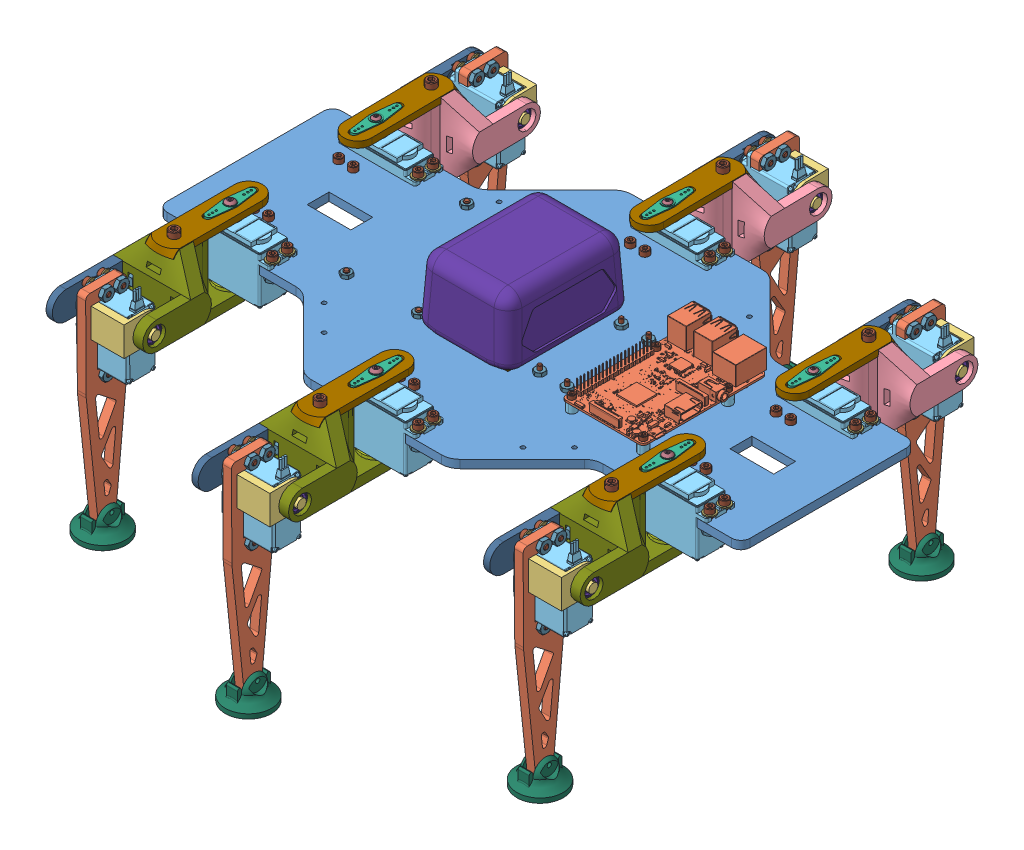
SolidWorks assembly Hexapod, configuration Défaut. Lengths in mm.
Overall size (400 185.52 400.76).
383 component instances, 23 part files, 135 mates.
Components (placement in the parent):
- Body-1: Body [Default] at (-400 -5.6 40) x (1 0 0) z (0 1 0) size (400 220 5.6)
- Leg_(Straight_Foot)-1: Leg_(Straight_Foot) [Default] at (-69.94 -26.67 -0.094) size (71.12 162.26 125.96)
  - Foot_(Straight)-1: Foot_(Straight) [Default] at (4.9357 4.6699 -91.3683) x (0.014203 -0.004158 0.99989) z (-0.999899 0 0.014203) size (28 145.4 6)
  - bearing_mount_foot-1: bearing_mount_foot [Default] at (4.8169 16.6428 -99.7277) x (-0.014203 0.004158 -0.99989) z (0.999899 0 -0.014203) size (25 20 29.5)
  - Joint-1: Joint [Défaut] at (35.768 26.4662 -54.7315) x (-0.014203 0 -0.999899) z (0 1 0) size (96.52 53.26 53.26)
  - hs-422-2: hs-422 [Défaut] at (5.1023 6.6131 -77.4551) x (-0.014203 0.004158 -0.99989) z (0.000059 0.999991 0.004158) size (19.81 42.09 58.23)
  - hs-422-3: hs-422 [Défaut] at (19.939 20.701 -19.812) x (0 0 1) z (-1 0 0) size (19.81 42.09 58.23)
  - hs-422_horn_straight-1: hs-422_horn_straight [Default] at (-16.9088 16.9412 -87.0065) x (0.014203 0 0.999899) z (0 1 0) size (33.93 4.93 8.79)
  - hs-422_horn_straight-2: hs-422_horn_straight [Default] at (9.652 42.5743 -9.906) x (-0.014203 0 -0.999899) z (-0.999899 0 0.014203) size (33.93 4.93 8.79)
  - Bearing_mount_leg-1: Bearing_mount_leg [Default] at (9.652 21 2.594) x (0 0 1) z (0 -1 0) size (35 20 30)
  - Bearing-1: Bearing [Default] at (9.652 -6.7498 -9.906) x (0.84763 0 0.530588) z (-0.530588 0 0.84763) size (13.87 4.75 13.87)
  - Bearing-2: Bearing [Default] at (32.2403 16.9412 -87.7047) x (0.007588 -0.845349 0.534161) z (-0.012007 -0.534214 -0.845264) size (13.87 4.75 13.87)
  - Joint_attachment_leg-1: Joint_attachment_leg [Défaut] at (35.768 26.4662 -54.7315) x (-0.014203 0 -0.999899) z (0 1 0) size (74.32 19.07 4.32)
  - Joint_attachment_foot-1: Joint_attachment_foot [Défaut] at (35.768 26.4662 -54.7315) x (-0.014203 0 -0.999899) z (0 1 0) size (64.08 6.7 19.07)
  - socket_1_2_6-32_with_washer-1: socket_1_2_6-32_with_washer [Défaut] at (43.4196 -14.698 -83.8589) x (0.999899 0 -0.014203) z (0.012271 -0.503597 0.863852) size (16.21 7.92 7.92)
    - socket head cap screw_ai-1: socket head cap screw_ai [HX-SHCS 0.138-32x0.5x0.5-N] at (-51.206 -1.62 2.0257) size (16.21 5.74 5.74)
    - flat washer type b narrow_ai-1: flat washer type b narrow_ai [Narrow FW 0.138] at (-46.888 -1.62 2.0257) size (0.81 7.92 7.92)
  - socket_1_2_6-32_with_washer-2: socket_1_2_6-32_with_washer [Défaut] at (43.2654 -19.0943 -94.7118) x (0.999899 0 -0.014203) z (0.000059 0.999991 0.004158) size (16.21 7.92 7.92)
    - socket head cap screw_ai-1: socket head cap screw_ai [HX-SHCS 0.138-32x0.5x0.5-N] at (-51.206 -1.62 2.0257) size (16.21 5.74 5.74)
    - flat washer type b narrow_ai-1: flat washer type b narrow_ai [Narrow FW 0.138] at (-46.888 -1.62 2.0257) size (0.81 7.92 7.92)
  - socket_1_2_6-32_with_washer-3: socket_1_2_6-32_with_washer [Défaut] at (43.4489 27.9623 -81.7931) x (0.999899 0 -0.014203) z (-0.012271 0.503597 -0.863852) size (16.21 7.92 7.92)
    - socket head cap screw_ai-1: socket head cap screw_ai [HX-SHCS 0.138-32x0.5x0.5-N] at (-51.206 -1.62 2.0257) size (16.21 5.74 5.74)
    - flat washer type b narrow_ai-1: flat washer type b narrow_ai [Narrow FW 0.138] at (-46.888 -1.62 2.0257) size (0.81 7.92 7.92)
  - socket_1_2_6-32_with_washer-4: socket_1_2_6-32_with_washer [Défaut] at (43.3046 28.0045 -91.952) x (0.999899 0 -0.014203) z (-0.012271 0.503597 -0.863852) size (16.21 7.92 7.92)
    - socket head cap screw_ai-1: socket head cap screw_ai [HX-SHCS 0.138-32x0.5x0.5-N] at (-51.206 -1.62 2.0257) size (16.21 5.74 5.74)
    - flat washer type b narrow_ai-1: flat washer type b narrow_ai [Narrow FW 0.138] at (-46.888 -1.62 2.0257) size (0.81 7.92 7.92)
  - socket button head cap screw_ai-2: socket button head cap screw_ai [SBHCSCREW 0.112-40x0.25-HX-N] at (-19.9057 16.9412 -86.964) x (0.999899 0 -0.014203) z (-0.007102 0.866025 -0.49995) size (7.85 5.41 5.41)
  - socket button head cap screw_ai-3: socket button head cap screw_ai [SBHCSCREW 0.112-40x0.25-HX-N] at (9.652 45.5715 -9.906) x (0 -1 0) z (0.87304 0 0.487649) size (7.85 5.41 5.41)
  - machine screw nut hex_ai-7: machine screw nut hex_ai [MSHXNUT 0.138-32-D-N] at (5.0634 -17.1176 -82.3797) x (0.01233 0.496395 0.868009) z (-0.999899 0 0.014203) size (7.92 9.15 2.9)
  - machine screw nut hex_ai-8: machine screw nut hex_ai [MSHXNUT 0.138-32-D-N] at (4.9191 -17.0754 -92.5386) x (-0.012271 0.503597 -0.863852) z (-0.999899 0 0.014203) size (7.92 9.15 2.9)
  - machine screw nut hex_ai-9: machine screw nut hex_ai [MSHXNUT 0.138-32-D-N] at (5.0662 30.382 -82.1822) x (0.000059 0.999991 0.004158) z (-0.999899 0 0.014203) size (7.92 9.15 2.9)
  - machine screw nut hex_ai-10: machine screw nut hex_ai [MSHXNUT 0.138-32-D-N] at (4.9219 30.4242 -92.3411) x (0.000059 0.999991 0.004158) z (-0.999899 0 0.014203) size (7.92 9.15 2.9)
  - socket head cap screw_ai-1: socket head cap screw_ai [HX-SHCS 0.164-32x0.5x0.5-N] at (9.1052 47.8568 -48.4) x (0 -1 0) z (0.014203 0 0.999899) size (16.87 6.86 6.86)
  - socket head cap screw_ai-2: socket head cap screw_ai [HX-SHCS 0.164-32x0.5x0.5-N] at (-21.967 16.9412 -59.205) x (0.999899 0 -0.014203) z (0.014203 0 0.999899) size (16.87 6.86 6.86)
  - machine screw nut hex_ai-11: machine screw nut hex_ai [MSHXNUT 0.164-32-D-N] at (9.1052 33.127 -48.4) x (0.87304 0 0.487649) z (0 1 0) size (8.74 10.09 3.3)
  - machine screw nut hex_ai-12: machine screw nut hex_ai [MSHXNUT 0.164-32-D-N] at (-7.2387 16.9412 -59.4142) x (0.014203 0 0.999899) z (-0.999899 0 0.014203) size (8.74 10.09 3.3)
  - socket head cap screw_ai-3: socket head cap screw_ai [HX-SHCS 0.112-40x0.5x0.5-N] at (-4.0273 11.7048 -99.6226) x (0.999899 0 -0.014203) z (0.014203 -0.004158 0.99989) size (15.54 4.65 4.65)
  - socket head cap screw_ai-4: socket head cap screw_ai [HX-SHCS 0.112-40x0.5x0.5-N] at (-4.0267 21.7048 -99.5811) x (0.999899 0 -0.014203) z (-0.014203 0.004158 -0.99989) size (15.54 4.65 4.65)
  - socket_1_2_6-32_with_washer-5: socket_1_2_6-32_with_washer [Défaut] at (-3.4199 -17.7034 -7.3903) x (0 -1 0) z (0.5 0 0.866025) size (16.21 7.92 7.92)
    - socket head cap screw_ai-1: socket head cap screw_ai [HX-SHCS 0.138-32x0.5x0.5-N] at (-51.206 -1.62 2.0257) size (16.21 5.74 5.74)
    - flat washer type b narrow_ai-1: flat washer type b narrow_ai [Narrow FW 0.138] at (-46.888 -1.62 2.0257) size (0.81 7.92 7.92)
  - socket_1_2_6-32_with_washer-6: socket_1_2_6-32_with_washer [Défaut] at (44.0781 -17.7034 -17.5503) x (0 -1 0) z (0.5 0 0.866025) size (16.21 7.92 7.92)
    - socket head cap screw_ai-1: socket head cap screw_ai [HX-SHCS 0.138-32x0.5x0.5-N] at (-51.206 -1.62 2.0257) size (16.21 5.74 5.74)
    - flat washer type b narrow_ai-1: flat washer type b narrow_ai [Narrow FW 0.138] at (-46.888 -1.62 2.0257) size (0.81 7.92 7.92)
  - socket_1_2_6-32_with_washer-7: socket_1_2_6-32_with_washer [Défaut] at (-3.4199 -17.7034 -17.5503) x (0 -1 0) z (0.5 0 0.866025) size (16.21 7.92 7.92)
    - socket head cap screw_ai-1: socket head cap screw_ai [HX-SHCS 0.138-32x0.5x0.5-N] at (-51.206 -1.62 2.0257) size (16.21 5.74 5.74)
    - flat washer type b narrow_ai-1: flat washer type b narrow_ai [Narrow FW 0.138] at (-46.888 -1.62 2.0257) size (0.81 7.92 7.92)
  - socket_1_2_6-32_with_washer-8: socket_1_2_6-32_with_washer [Défaut] at (44.0781 -17.7034 -7.3903) x (0 -1 0) z (0.5 0 0.866025) size (16.21 7.92 7.92)
    - socket head cap screw_ai-1: socket head cap screw_ai [HX-SHCS 0.138-32x0.5x0.5-N] at (-51.206 -1.62 2.0257) size (16.21 5.74 5.74)
    - flat washer type b narrow_ai-1: flat washer type b narrow_ai [Narrow FW 0.138] at (-46.888 -1.62 2.0257) size (0.81 7.92 7.92)
  - Slippers-1: Slippers [Default] at (1.9298 -111.2299 -91.7597) x (0.999899 0 -0.014203) z (0.014203 0 0.999899) size (35.48 18.25 37.71)
- Leg_(Straight_Foot)-2: Leg_(Straight_Foot) [Default] at (-369.94 -26.67 -0.094) size (71.12 162.26 125.96)
  - Foot_(Straight)-1: Foot_(Straight) [Default] at (4.9357 4.6699 -91.3683) x (0.014203 -0.004158 0.99989) z (-0.999899 0 0.014203) size (28 145.4 6)
  - bearing_mount_foot-1: bearing_mount_foot [Default] at (4.8169 16.6428 -99.7277) x (-0.014203 0.004158 -0.99989) z (0.999899 0 -0.014203) size (25 20 29.5)
  - Joint-1: Joint [Défaut] at (35.768 26.4662 -54.7315) x (-0.014203 0 -0.999899) z (0 1 0) size (96.52 53.26 53.26)
  - hs-422-2: hs-422 [Défaut] at (5.1023 6.6131 -77.4551) x (-0.014203 0.004158 -0.99989) z (0.000059 0.999991 0.004158) size (19.81 42.09 58.23)
  - hs-422-3: hs-422 [Défaut] at (19.939 20.701 -19.812) x (0 0 1) z (-1 0 0) size (19.81 42.09 58.23)
  - hs-422_horn_straight-1: hs-422_horn_straight [Default] at (-16.9088 16.9412 -87.0065) x (0.014203 0 0.999899) z (0 1 0) size (33.93 4.93 8.79)
  - hs-422_horn_straight-2: hs-422_horn_straight [Default] at (9.652 42.5743 -9.906) x (-0.014203 0 -0.999899) z (-0.999899 0 0.014203) size (33.93 4.93 8.79)
  - Bearing_mount_leg-1: Bearing_mount_leg [Default] at (9.652 21 2.594) x (0 0 1) z (0 -1 0) size (35 20 30)
  - Bearing-1: Bearing [Default] at (9.652 -6.7498 -9.906) x (0.84763 0 0.530588) z (-0.530588 0 0.84763) size (13.87 4.75 13.87)
  - Bearing-2: Bearing [Default] at (32.2403 16.9412 -87.7047) x (0.007588 -0.845349 0.534161) z (-0.012007 -0.534214 -0.845264) size (13.87 4.75 13.87)
  - Joint_attachment_leg-1: Joint_attachment_leg [Défaut] at (35.768 26.4662 -54.7315) x (-0.014203 0 -0.999899) z (0 1 0) size (74.32 19.07 4.32)
  - Joint_attachment_foot-1: Joint_attachment_foot [Défaut] at (35.768 26.4662 -54.7315) x (-0.014203 0 -0.999899) z (0 1 0) size (64.08 6.7 19.07)
  - socket_1_2_6-32_with_washer-1: socket_1_2_6-32_with_washer [Défaut] at (43.4196 -14.698 -83.8589) x (0.999899 0 -0.014203) z (0.012271 -0.503597 0.863852) size (16.21 7.92 7.92)
    - socket head cap screw_ai-1: socket head cap screw_ai [HX-SHCS 0.138-32x0.5x0.5-N] at (-51.206 -1.62 2.0257) size (16.21 5.74 5.74)
    - flat washer type b narrow_ai-1: flat washer type b narrow_ai [Narrow FW 0.138] at (-46.888 -1.62 2.0257) size (0.81 7.92 7.92)
  - socket_1_2_6-32_with_washer-2: socket_1_2_6-32_with_washer [Défaut] at (43.2654 -19.0943 -94.7118) x (0.999899 0 -0.014203) z (0.000059 0.999991 0.004158) size (16.21 7.92 7.92)
    - socket head cap screw_ai-1: socket head cap screw_ai [HX-SHCS 0.138-32x0.5x0.5-N] at (-51.206 -1.62 2.0257) size (16.21 5.74 5.74)
    - flat washer type b narrow_ai-1: flat washer type b narrow_ai [Narrow FW 0.138] at (-46.888 -1.62 2.0257) size (0.81 7.92 7.92)
  - socket_1_2_6-32_with_washer-3: socket_1_2_6-32_with_washer [Défaut] at (43.4489 27.9623 -81.7931) x (0.999899 0 -0.014203) z (-0.012271 0.503597 -0.863852) size (16.21 7.92 7.92)
    - socket head cap screw_ai-1: socket head cap screw_ai [HX-SHCS 0.138-32x0.5x0.5-N] at (-51.206 -1.62 2.0257) size (16.21 5.74 5.74)
    - flat washer type b narrow_ai-1: flat washer type b narrow_ai [Narrow FW 0.138] at (-46.888 -1.62 2.0257) size (0.81 7.92 7.92)
  - socket_1_2_6-32_with_washer-4: socket_1_2_6-32_with_washer [Défaut] at (43.3046 28.0045 -91.952) x (0.999899 0 -0.014203) z (-0.012271 0.503597 -0.863852) size (16.21 7.92 7.92)
    - socket head cap screw_ai-1: socket head cap screw_ai [HX-SHCS 0.138-32x0.5x0.5-N] at (-51.206 -1.62 2.0257) size (16.21 5.74 5.74)
    - flat washer type b narrow_ai-1: flat washer type b narrow_ai [Narrow FW 0.138] at (-46.888 -1.62 2.0257) size (0.81 7.92 7.92)
  - socket button head cap screw_ai-2: socket button head cap screw_ai [SBHCSCREW 0.112-40x0.25-HX-N] at (-19.9057 16.9412 -86.964) x (0.999899 0 -0.014203) z (-0.007102 0.866025 -0.49995) size (7.85 5.41 5.41)
  - socket button head cap screw_ai-3: socket button head cap screw_ai [SBHCSCREW 0.112-40x0.25-HX-N] at (9.652 45.5715 -9.906) x (0 -1 0) z (0.87304 0 0.487649) size (7.85 5.41 5.41)
  - machine screw nut hex_ai-7: machine screw nut hex_ai [MSHXNUT 0.138-32-D-N] at (5.0634 -17.1176 -82.3797) x (0.01233 0.496395 0.868009) z (-0.999899 0 0.014203) size (7.92 9.15 2.9)
  - machine screw nut hex_ai-8: machine screw nut hex_ai [MSHXNUT 0.138-32-D-N] at (4.9191 -17.0754 -92.5386) x (-0.012271 0.503597 -0.863852) z (-0.999899 0 0.014203) size (7.92 9.15 2.9)
  - machine screw nut hex_ai-9: machine screw nut hex_ai [MSHXNUT 0.138-32-D-N] at (5.0662 30.382 -82.1822) x (0.000059 0.999991 0.004158) z (-0.999899 0 0.014203) size (7.92 9.15 2.9)
  - machine screw nut hex_ai-10: machine screw nut hex_ai [MSHXNUT 0.138-32-D-N] at (4.9219 30.4242 -92.3411) x (0.000059 0.999991 0.004158) z (-0.999899 0 0.014203) size (7.92 9.15 2.9)
  - socket head cap screw_ai-1: socket head cap screw_ai [HX-SHCS 0.164-32x0.5x0.5-N] at (9.1052 47.8568 -48.4) x (0 -1 0) z (0.014203 0 0.999899) size (16.87 6.86 6.86)
  - socket head cap screw_ai-2: socket head cap screw_ai [HX-SHCS 0.164-32x0.5x0.5-N] at (-21.967 16.9412 -59.205) x (0.999899 0 -0.014203) z (0.014203 0 0.999899) size (16.87 6.86 6.86)
  - machine screw nut hex_ai-11: machine screw nut hex_ai [MSHXNUT 0.164-32-D-N] at (9.1052 33.127 -48.4) x (0.87304 0 0.487649) z (0 1 0) size (8.74 10.09 3.3)
  - machine screw nut hex_ai-12: machine screw nut hex_ai [MSHXNUT 0.164-32-D-N] at (-7.2387 16.9412 -59.4142) x (0.014203 0 0.999899) z (-0.999899 0 0.014203) size (8.74 10.09 3.3)
  - socket head cap screw_ai-3: socket head cap screw_ai [HX-SHCS 0.112-40x0.5x0.5-N] at (-4.0273 11.7048 -99.6226) x (0.999899 0 -0.014203) z (0.014203 -0.004158 0.99989) size (15.54 4.65 4.65)
  - socket head cap screw_ai-4: socket head cap screw_ai [HX-SHCS 0.112-40x0.5x0.5-N] at (-4.0267 21.7048 -99.5811) x (0.999899 0 -0.014203) z (-0.014203 0.004158 -0.99989) size (15.54 4.65 4.65)
  - socket_1_2_6-32_with_washer-5: socket_1_2_6-32_with_washer [Défaut] at (-3.4199 -17.7034 -7.3903) x (0 -1 0) z (0.5 0 0.866025) size (16.21 7.92 7.92)
    - socket head cap screw_ai-1: socket head cap screw_ai [HX-SHCS 0.138-32x0.5x0.5-N] at (-51.206 -1.62 2.0257) size (16.21 5.74 5.74)
    - flat washer type b narrow_ai-1: flat washer type b narrow_ai [Narrow FW 0.138] at (-46.888 -1.62 2.0257) size (0.81 7.92 7.92)
  - socket_1_2_6-32_with_washer-6: socket_1_2_6-32_with_washer [Défaut] at (44.0781 -17.7034 -17.5503) x (0 -1 0) z (0.5 0 0.866025) size (16.21 7.92 7.92)
    - socket head cap screw_ai-1: socket head cap screw_ai [HX-SHCS 0.138-32x0.5x0.5-N] at (-51.206 -1.62 2.0257) size (16.21 5.74 5.74)
    - flat washer type b narrow_ai-1: flat washer type b narrow_ai [Narrow FW 0.138] at (-46.888 -1.62 2.0257) size (0.81 7.92 7.92)
  - socket_1_2_6-32_with_washer-7: socket_1_2_6-32_with_washer [Défaut] at (-3.4199 -17.7034 -17.5503) x (0 -1 0) z (0.5 0 0.866025) size (16.21 7.92 7.92)
    - socket head cap screw_ai-1: socket head cap screw_ai [HX-SHCS 0.138-32x0.5x0.5-N] at (-51.206 -1.62 2.0257) size (16.21 5.74 5.74)
    - flat washer type b narrow_ai-1: flat washer type b narrow_ai [Narrow FW 0.138] at (-46.888 -1.62 2.0257) size (0.81 7.92 7.92)
  - socket_1_2_6-32_with_washer-8: socket_1_2_6-32_with_washer [Défaut] at (44.0781 -17.7034 -7.3903) x (0 -1 0) z (0.5 0 0.866025) size (16.21 7.92 7.92)
    - socket head cap screw_ai-1: socket head cap screw_ai [HX-SHCS 0.138-32x0.5x0.5-N] at (-51.206 -1.62 2.0257) size (16.21 5.74 5.74)
    - flat washer type b narrow_ai-1: flat washer type b narrow_ai [Narrow FW 0.138] at (-46.888 -1.62 2.0257) size (0.81 7.92 7.92)
  - Slippers-1: Slippers [Default] at (1.9298 -111.2299 -91.7597) x (0.999899 0 -0.014203) z (0.014203 0 0.999899) size (35.48 18.25 37.71)
- Leg_(Straight_Foot)-3: Leg_(Straight_Foot) [Default] at (-219.94 -26.67 -50.094) size (71.12 162.26 125.96)
  - Foot_(Straight)-1: Foot_(Straight) [Default] at (4.9357 4.6699 -91.3683) x (0.014203 -0.004158 0.99989) z (-0.999899 0 0.014203) size (28 145.4 6)
  - bearing_mount_foot-1: bearing_mount_foot [Default] at (4.8169 16.6428 -99.7277) x (-0.014203 0.004158 -0.99989) z (0.999899 0 -0.014203) size (25 20 29.5)
  - Joint-1: Joint [Défaut] at (35.768 26.4662 -54.7315) x (-0.014203 0 -0.999899) z (0 1 0) size (96.52 53.26 53.26)
  - hs-422-2: hs-422 [Défaut] at (5.1023 6.6131 -77.4551) x (-0.014203 0.004158 -0.99989) z (0.000059 0.999991 0.004158) size (19.81 42.09 58.23)
  - hs-422-3: hs-422 [Défaut] at (19.939 20.701 -19.812) x (0 0 1) z (-1 0 0) size (19.81 42.09 58.23)
  - hs-422_horn_straight-1: hs-422_horn_straight [Default] at (-16.9088 16.9412 -87.0065) x (0.014203 0 0.999899) z (0 1 0) size (33.93 4.93 8.79)
  - hs-422_horn_straight-2: hs-422_horn_straight [Default] at (9.652 42.5743 -9.906) x (-0.014203 0 -0.999899) z (-0.999899 0 0.014203) size (33.93 4.93 8.79)
  - Bearing_mount_leg-1: Bearing_mount_leg [Default] at (9.652 21 2.594) x (0 0 1) z (0 -1 0) size (35 20 30)
  - Bearing-1: Bearing [Default] at (9.652 -6.7498 -9.906) x (0.84763 0 0.530588) z (-0.530588 0 0.84763) size (13.87 4.75 13.87)
  - Bearing-2: Bearing [Default] at (32.2403 16.9412 -87.7047) x (0.007588 -0.845349 0.534161) z (-0.012007 -0.534214 -0.845264) size (13.87 4.75 13.87)
  - Joint_attachment_leg-1: Joint_attachment_leg [Défaut] at (35.768 26.4662 -54.7315) x (-0.014203 0 -0.999899) z (0 1 0) size (74.32 19.07 4.32)
  - Joint_attachment_foot-1: Joint_attachment_foot [Défaut] at (35.768 26.4662 -54.7315) x (-0.014203 0 -0.999899) z (0 1 0) size (64.08 6.7 19.07)
  - socket_1_2_6-32_with_washer-1: socket_1_2_6-32_with_washer [Défaut] at (43.4196 -14.698 -83.8589) x (0.999899 0 -0.014203) z (0.012271 -0.503597 0.863852) size (16.21 7.92 7.92)
    - socket head cap screw_ai-1: socket head cap screw_ai [HX-SHCS 0.138-32x0.5x0.5-N] at (-51.206 -1.62 2.0257) size (16.21 5.74 5.74)
    - flat washer type b narrow_ai-1: flat washer type b narrow_ai [Narrow FW 0.138] at (-46.888 -1.62 2.0257) size (0.81 7.92 7.92)
  - socket_1_2_6-32_with_washer-2: socket_1_2_6-32_with_washer [Défaut] at (43.2654 -19.0943 -94.7118) x (0.999899 0 -0.014203) z (0.000059 0.999991 0.004158) size (16.21 7.92 7.92)
    - socket head cap screw_ai-1: socket head cap screw_ai [HX-SHCS 0.138-32x0.5x0.5-N] at (-51.206 -1.62 2.0257) size (16.21 5.74 5.74)
    - flat washer type b narrow_ai-1: flat washer type b narrow_ai [Narrow FW 0.138] at (-46.888 -1.62 2.0257) size (0.81 7.92 7.92)
  - socket_1_2_6-32_with_washer-3: socket_1_2_6-32_with_washer [Défaut] at (43.4489 27.9623 -81.7931) x (0.999899 0 -0.014203) z (-0.012271 0.503597 -0.863852) size (16.21 7.92 7.92)
    - socket head cap screw_ai-1: socket head cap screw_ai [HX-SHCS 0.138-32x0.5x0.5-N] at (-51.206 -1.62 2.0257) size (16.21 5.74 5.74)
    - flat washer type b narrow_ai-1: flat washer type b narrow_ai [Narrow FW 0.138] at (-46.888 -1.62 2.0257) size (0.81 7.92 7.92)
  - socket_1_2_6-32_with_washer-4: socket_1_2_6-32_with_washer [Défaut] at (43.3046 28.0045 -91.952) x (0.999899 0 -0.014203) z (-0.012271 0.503597 -0.863852) size (16.21 7.92 7.92)
    - socket head cap screw_ai-1: socket head cap screw_ai [HX-SHCS 0.138-32x0.5x0.5-N] at (-51.206 -1.62 2.0257) size (16.21 5.74 5.74)
    - flat washer type b narrow_ai-1: flat washer type b narrow_ai [Narrow FW 0.138] at (-46.888 -1.62 2.0257) size (0.81 7.92 7.92)
  - socket button head cap screw_ai-2: socket button head cap screw_ai [SBHCSCREW 0.112-40x0.25-HX-N] at (-19.9057 16.9412 -86.964) x (0.999899 0 -0.014203) z (-0.007102 0.866025 -0.49995) size (7.85 5.41 5.41)
  - socket button head cap screw_ai-3: socket button head cap screw_ai [SBHCSCREW 0.112-40x0.25-HX-N] at (9.652 45.5715 -9.906) x (0 -1 0) z (0.87304 0 0.487649) size (7.85 5.41 5.41)
  - machine screw nut hex_ai-7: machine screw nut hex_ai [MSHXNUT 0.138-32-D-N] at (5.0634 -17.1176 -82.3797) x (0.01233 0.496395 0.868009) z (-0.999899 0 0.014203) size (7.92 9.15 2.9)
  - machine screw nut hex_ai-8: machine screw nut hex_ai [MSHXNUT 0.138-32-D-N] at (4.9191 -17.0754 -92.5386) x (-0.012271 0.503597 -0.863852) z (-0.999899 0 0.014203) size (7.92 9.15 2.9)
  - machine screw nut hex_ai-9: machine screw nut hex_ai [MSHXNUT 0.138-32-D-N] at (5.0662 30.382 -82.1822) x (0.000059 0.999991 0.004158) z (-0.999899 0 0.014203) size (7.92 9.15 2.9)
  - machine screw nut hex_ai-10: machine screw nut hex_ai [MSHXNUT 0.138-32-D-N] at (4.9219 30.4242 -92.3411) x (0.000059 0.999991 0.004158) z (-0.999899 0 0.014203) size (7.92 9.15 2.9)
  - socket head cap screw_ai-1: socket head cap screw_ai [HX-SHCS 0.164-32x0.5x0.5-N] at (9.1052 47.8568 -48.4) x (0 -1 0) z (0.014203 0 0.999899) size (16.87 6.86 6.86)
  - socket head cap screw_ai-2: socket head cap screw_ai [HX-SHCS 0.164-32x0.5x0.5-N] at (-21.967 16.9412 -59.205) x (0.999899 0 -0.014203) z (0.014203 0 0.999899) size (16.87 6.86 6.86)
  - machine screw nut hex_ai-11: machine screw nut hex_ai [MSHXNUT 0.164-32-D-N] at (9.1052 33.127 -48.4) x (0.87304 0 0.487649) z (0 1 0) size (8.74 10.09 3.3)
  - machine screw nut hex_ai-12: machine screw nut hex_ai [MSHXNUT 0.164-32-D-N] at (-7.2387 16.9412 -59.4142) x (0.014203 0 0.999899) z (-0.999899 0 0.014203) size (8.74 10.09 3.3)
  - socket head cap screw_ai-3: socket head cap screw_ai [HX-SHCS 0.112-40x0.5x0.5-N] at (-4.0273 11.7048 -99.6226) x (0.999899 0 -0.014203) z (0.014203 -0.004158 0.99989) size (15.54 4.65 4.65)
  - socket head cap screw_ai-4: socket head cap screw_ai [HX-SHCS 0.112-40x0.5x0.5-N] at (-4.0267 21.7048 -99.5811) x (0.999899 0 -0.014203) z (-0.014203 0.004158 -0.99989) size (15.54 4.65 4.65)
  - socket_1_2_6-32_with_washer-5: socket_1_2_6-32_with_washer [Défaut] at (-3.4199 -17.7034 -7.3903) x (0 -1 0) z (0.5 0 0.866025) size (16.21 7.92 7.92)
    - socket head cap screw_ai-1: socket head cap screw_ai [HX-SHCS 0.138-32x0.5x0.5-N] at (-51.206 -1.62 2.0257) size (16.21 5.74 5.74)
    - flat washer type b narrow_ai-1: flat washer type b narrow_ai [Narrow FW 0.138] at (-46.888 -1.62 2.0257) size (0.81 7.92 7.92)
  - socket_1_2_6-32_with_washer-6: socket_1_2_6-32_with_washer [Défaut] at (44.0781 -17.7034 -17.5503) x (0 -1 0) z (0.5 0 0.866025) size (16.21 7.92 7.92)
    - socket head cap screw_ai-1: socket head cap screw_ai [HX-SHCS 0.138-32x0.5x0.5-N] at (-51.206 -1.62 2.0257) size (16.21 5.74 5.74)
    - flat washer type b narrow_ai-1: flat washer type b narrow_ai [Narrow FW 0.138] at (-46.888 -1.62 2.0257) size (0.81 7.92 7.92)
  - socket_1_2_6-32_with_washer-7: socket_1_2_6-32_with_washer [Défaut] at (-3.4199 -17.7034 -17.5503) x (0 -1 0) z (0.5 0 0.866025) size (16.21 7.92 7.92)
    - socket head cap screw_ai-1: socket head cap screw_ai [HX-SHCS 0.138-32x0.5x0.5-N] at (-51.206 -1.62 2.0257) size (16.21 5.74 5.74)
    - flat washer type b narrow_ai-1: flat washer type b narrow_ai [Narrow FW 0.138] at (-46.888 -1.62 2.0257) size (0.81 7.92 7.92)
  - socket_1_2_6-32_with_washer-8: socket_1_2_6-32_with_washer [Défaut] at (44.0781 -17.7034 -7.3903) x (0 -1 0) z (0.5 0 0.866025) size (16.21 7.92 7.92)
    - socket head cap screw_ai-1: socket head cap screw_ai [HX-SHCS 0.138-32x0.5x0.5-N] at (-51.206 -1.62 2.0257) size (16.21 5.74 5.74)
    - flat washer type b narrow_ai-1: flat washer type b narrow_ai [Narrow FW 0.138] at (-46.888 -1.62 2.0257) size (0.81 7.92 7.92)
  - Slippers-1: Slippers [Default] at (1.9298 -111.2299 -91.7597) x (0.999899 0 -0.014203) z (0.014203 0 0.999899) size (35.48 18.25 37.71)
- Leg_(Straight_Foot)_(Mirror)-1: Leg_(Straight_Foot)_(Mirror) [Default] at (-369.94 -26.67 99.906) size (70.34 162.3 124.8)
  - Joint_(Mirror)-1: Joint_(Mirror) [Défaut] at (36.4933 -51.1276 34.4889) x (0.002055 0 0.999998) z (0 -1 0) size (96.52 53.26 53.26)
  - hs-422-3: hs-422 [Défaut] at (19.939 20.701 -19.812) x (0 0 1) z (-1 0 0) size (19.81 42.09 58.23)
  - hs-422_horn_straight-2: hs-422_horn_straight [Default] at (9.652 42.5743 -9.906) x (0.002055 0 0.999998) z (0.999998 0 -0.002055) size (33.93 4.93 8.79)
  - Bearing_mount_leg-1: Bearing_mount_leg [Default] at (9.652 21 -22.406) x (0 0 -1) z (0 -1 0) size (35 20 30)
  - Bearing-1: Bearing [Default] at (9.652 -6.7498 -9.906) x (0.266287 0 0.963894) z (-0.963894 0 0.266287) size (13.87 4.75 13.87)
  - Joint_attachment_leg-1: Joint_attachment_leg [Défaut] at (-17.0066 26.5024 34.5989) x (0.002055 0 0.999998) z (0 1 0) size (74.32 19.07 4.32)
  - bearing_mount_foot-2: bearing_mount_foot [Default] at (6.7141 17.2663 79.9818) x (0.002055 -0.004919 0.999986) z (0.999998 0 -0.002055) size (25 20 29.5)
  - Bearing-3: Bearing [Default] at (29.1886 16.9774 67.524) x (-0.001098 -0.845349 -0.534213) z (0.001738 -0.534214 0.845347) size (13.87 4.75 13.87)
  - hs-422-4: hs-422 [Défaut] at (6.0779 6.6418 77.4268) x (-0.002055 0.004919 -0.999986) z (0.00001 0.999988 0.004919) size (19.81 42.09 58.23)
  - hs-422_horn_straight-3: hs-422_horn_straight [Default] at (-15.8156 16.9774 67.6165) x (-0.002055 0 -0.999998) z (0 -1 0) size (33.93 4.93 8.79)
  - Foot_(Straight)-2: Foot_(Straight) [Default] at (0.0967 4.6719 71.5233) x (-0.002055 0.004919 -0.999986) z (0.999998 0 -0.002055) size (28 145.4 6)
  - Joint_attachment_foot-2: Joint_attachment_foot [Défaut] at (36.4933 7.4524 34.4889) x (0.002055 0 0.999998) z (0 -1 0) size (64.08 6.7 19.07)
  - socket button head cap screw_ai-1: socket button head cap screw_ai [SBHCSCREW 0.138-32x0.25-HX-N] at (-19.1684 16.9774 67.6234) x (0.999998 0 -0.002055) z (0.002055 0 0.999998) size (8.2 6.65 6.65)
  - socket button head cap screw_ai-2: socket button head cap screw_ai [SBHCSCREW 0.138-32x0.25-HX-N] at (9.652 45.9271 -9.906) x (0 -1 0) z (-0.864996 0 0.501779) size (8.2 6.65 6.65)
  - socket head cap screw_ai-1: socket head cap screw_ai [HX-SHCS 0.112-40x0.5x0.5-N] at (-2.7306 21.6303 80.0227) x (0.999998 0 -0.002055) z (0.001019 -0.868474 0.495733) size (15.54 4.65 4.65)
  - socket head cap screw_ai-2: socket head cap screw_ai [HX-SHCS 0.112-40x0.5x0.5-N] at (-2.7307 11.6304 79.9735) x (0.999998 0 -0.002055) z (0.001036 0.863555 0.504253) size (15.54 4.65 4.65)
  - socket head cap screw_ai-3: socket head cap screw_ai [HX-SHCS 0.164-32x0.5x0.5-N] at (-21.1613 16.9774 39.9006) x (0.999998 0 -0.002055) z (0.001028 0.866025 0.499999) size (16.87 6.86 6.86)
  - socket head cap screw_ai-4: socket head cap screw_ai [HX-SHCS 0.164-32x0.5x0.5-N] at (9.7311 47.893 28.5918) x (0 -1 0) z (0.002055 0 0.999998) size (16.87 6.86 6.86)
  - socket_1_2_6-32_with_washer-1: socket_1_2_6-32_with_washer [Défaut] at (44.4497 32.8866 61.5465) x (0.999998 0 -0.002055) z (0.001775 -0.504254 0.863554) size (16.21 7.92 7.92)
    - socket head cap screw_ai-1: socket head cap screw_ai [HX-SHCS 0.138-32x0.5x0.5-N] at (-51.206 -1.62 2.0257) size (16.21 5.74 5.74)
    - flat washer type b narrow_ai-1: flat washer type b narrow_ai [Narrow FW 0.138] at (-46.888 -1.62 2.0257) size (0.81 7.92 7.92)
  - socket_1_2_6-32_with_washer-2: socket_1_2_6-32_with_washer [Défaut] at (44.4545 -15.0155 63.8752) x (0.999998 0 -0.002055) z (-0.00001 -0.999988 -0.004919) size (16.21 7.92 7.92)
    - socket head cap screw_ai-1: socket head cap screw_ai [HX-SHCS 0.138-32x0.5x0.5-N] at (-51.206 -1.62 2.0257) size (16.21 5.74 5.74)
    - flat washer type b narrow_ai-1: flat washer type b narrow_ai [Narrow FW 0.138] at (-46.888 -1.62 2.0257) size (0.81 7.92 7.92)
  - socket_1_2_6-32_with_washer-3: socket_1_2_6-32_with_washer [Défaut] at (44.4701 -14.6628 71.4727) x (0.999998 0 -0.002055) z (0.001775 -0.504254 0.863554) size (16.21 7.92 7.92)
    - socket head cap screw_ai-1: socket head cap screw_ai [HX-SHCS 0.138-32x0.5x0.5-N] at (-51.206 -1.62 2.0257) size (16.21 5.74 5.74)
    - flat washer type b narrow_ai-1: flat washer type b narrow_ai [Narrow FW 0.138] at (-46.888 -1.62 2.0257) size (0.81 7.92 7.92)
  - socket_1_2_6-32_with_washer-4: socket_1_2_6-32_with_washer [Défaut] at (44.4706 32.8366 71.7064) x (0.999998 0 -0.002055) z (0.001775 -0.504254 0.863554) size (16.21 7.92 7.92)
    - socket head cap screw_ai-1: socket head cap screw_ai [HX-SHCS 0.138-32x0.5x0.5-N] at (-51.206 -1.62 2.0257) size (16.21 5.74 5.74)
    - flat washer type b narrow_ai-1: flat washer type b narrow_ai [Narrow FW 0.138] at (-46.888 -1.62 2.0257) size (0.81 7.92 7.92)
  - machine screw nut hex_ai-4: machine screw nut hex_ai [MSHXNUT 0.138-32-D-N] at (6.0779 -17.0332 62.3241) x (-0.001785 -0.495734 -0.868473) z (-0.999998 0 0.002055) size (7.92 9.15 2.9)
  - machine screw nut hex_ai-7: machine screw nut hex_ai [MSHXNUT 0.138-32-D-N] at (8.9943 -17.0832 72.478) x (-0.001775 0.504254 -0.863554) z (0.999998 0 -0.002055) size (7.92 9.15 2.9)
  - machine screw nut hex_ai-8: machine screw nut hex_ai [MSHXNUT 0.138-32-D-N] at (8.9739 30.4662 62.5518) x (0.00001 0.999988 0.004919) z (0.999998 0 -0.002055) size (7.92 9.15 2.9)
  - machine screw nut hex_ai-9: machine screw nut hex_ai [MSHXNUT 0.138-32-D-N] at (6.0992 30.4162 72.7176) x (-0.001785 -0.495734 -0.868473) z (-0.999998 0 0.002055) size (7.92 9.15 2.9)
  - socket_1_2_6-32_with_washer-5: socket_1_2_6-32_with_washer [Défaut] at (-3.4199 -17.7034 -7.3903) x (0 -1 0) z (0.5 0 0.866025) size (16.21 7.92 7.92)
    - socket head cap screw_ai-1: socket head cap screw_ai [HX-SHCS 0.138-32x0.5x0.5-N] at (-51.206 -1.62 2.0257) size (16.21 5.74 5.74)
    - flat washer type b narrow_ai-1: flat washer type b narrow_ai [Narrow FW 0.138] at (-46.888 -1.62 2.0257) size (0.81 7.92 7.92)
  - socket head cap screw_ai-5: socket head cap screw_ai [HX-SHCS 0.138-32x0.5x0.5-N] at (-3.81 33.5026 -14.986) x (0 -1 0) z (-1 0 0) size (16.21 5.74 5.74)
  - flat washer type b narrow_ai-1: flat washer type b narrow_ai [Narrow FW 0.138] at (-3.81 29.1846 -14.986) x (0 -1 0) z (0.546944 0 -0.837169) size (0.81 7.92 7.92)
  - socket head cap screw_ai-6: socket head cap screw_ai [HX-SHCS 0.138-32x0.5x0.5-N] at (43.688 33.5026 -14.986) x (0 -1 0) z (-1 0 0) size (16.21 5.74 5.74)
  - flat washer type b narrow_ai-2: flat washer type b narrow_ai [Narrow FW 0.138] at (43.688 29.1846 -14.986) x (0 -1 0) z (0.546944 0 -0.837169) size (0.81 7.92 7.92)
  - socket head cap screw_ai-7: socket head cap screw_ai [HX-SHCS 0.138-32x0.5x0.5-N] at (43.688 33.5026 -4.826) x (0 -1 0) z (-0.5 0 0.866025) size (16.21 5.74 5.74)
  - flat washer type b narrow_ai-3: flat washer type b narrow_ai [Narrow FW 0.138] at (43.688 29.1846 -4.826) x (0 -1 0) z (0.546944 0 -0.837169) size (0.81 7.92 7.92)
  - machine screw nut hex_ai-10: machine screw nut hex_ai [MSHXNUT 0.164-32-D-N] at (-6.4315 16.9774 39.8703) x (0.002055 0 0.999998) z (-0.999998 0 0.002055) size (8.74 10.09 3.3)
  - machine screw nut hex_ai-11: machine screw nut hex_ai [MSHXNUT 0.164-32-D-N] at (9.7311 29.8612 28.5918) x (-0.002055 0 -0.999998) z (0 -1 0) size (8.74 10.09 3.3)
  - Slippers-1: Slippers [Default] at (3.0957 -111.2276 71.0036) x (0.999998 0 -0.002055) z (0.002055 0 0.999998) size (35.48 18.25 37.71)
- Leg_(Straight_Foot)_(Mirror)-2: Leg_(Straight_Foot)_(Mirror) [Default] at (-69.94 -26.67 99.906) size (70.34 162.3 124.8)
  - Joint_(Mirror)-1: Joint_(Mirror) [Défaut] at (36.4933 -51.1276 34.4889) x (0.002055 0 0.999998) z (0 -1 0) size (96.52 53.26 53.26)
  - hs-422-3: hs-422 [Défaut] at (19.939 20.701 -19.812) x (0 0 1) z (-1 0 0) size (19.81 42.09 58.23)
  - hs-422_horn_straight-2: hs-422_horn_straight [Default] at (9.652 42.5743 -9.906) x (0.002055 0 0.999998) z (0.999998 0 -0.002055) size (33.93 4.93 8.79)
  - Bearing_mount_leg-1: Bearing_mount_leg [Default] at (9.652 21 -22.406) x (0 0 -1) z (0 -1 0) size (35 20 30)
  - Bearing-1: Bearing [Default] at (9.652 -6.7498 -9.906) x (0.266287 0 0.963894) z (-0.963894 0 0.266287) size (13.87 4.75 13.87)
  - Joint_attachment_leg-1: Joint_attachment_leg [Défaut] at (-17.0066 26.5024 34.5989) x (0.002055 0 0.999998) z (0 1 0) size (74.32 19.07 4.32)
  - bearing_mount_foot-2: bearing_mount_foot [Default] at (6.7141 17.2663 79.9818) x (0.002055 -0.004919 0.999986) z (0.999998 0 -0.002055) size (25 20 29.5)
  - Bearing-3: Bearing [Default] at (29.1886 16.9774 67.524) x (-0.001098 -0.845349 -0.534213) z (0.001738 -0.534214 0.845347) size (13.87 4.75 13.87)
  - hs-422-4: hs-422 [Défaut] at (6.0779 6.6418 77.4268) x (-0.002055 0.004919 -0.999986) z (0.00001 0.999988 0.004919) size (19.81 42.09 58.23)
  - hs-422_horn_straight-3: hs-422_horn_straight [Default] at (-15.8156 16.9774 67.6165) x (-0.002055 0 -0.999998) z (0 -1 0) size (33.93 4.93 8.79)
  - Foot_(Straight)-2: Foot_(Straight) [Default] at (0.0967 4.6719 71.5233) x (-0.002055 0.004919 -0.999986) z (0.999998 0 -0.002055) size (28 145.4 6)
  - Joint_attachment_foot-2: Joint_attachment_foot [Défaut] at (36.4933 7.4524 34.4889) x (0.002055 0 0.999998) z (0 -1 0) size (64.08 6.7 19.07)
  - socket button head cap screw_ai-1: socket button head cap screw_ai [SBHCSCREW 0.138-32x0.25-HX-N] at (-19.1684 16.9774 67.6234) x (0.999998 0 -0.002055) z (0.002055 0 0.999998) size (8.2 6.65 6.65)
  - socket button head cap screw_ai-2: socket button head cap screw_ai [SBHCSCREW 0.138-32x0.25-HX-N] at (9.652 45.9271 -9.906) x (0 -1 0) z (-0.864996 0 0.501779) size (8.2 6.65 6.65)
  - socket head cap screw_ai-1: socket head cap screw_ai [HX-SHCS 0.112-40x0.5x0.5-N] at (-2.7306 21.6303 80.0227) x (0.999998 0 -0.002055) z (0.001019 -0.868474 0.495733) size (15.54 4.65 4.65)
  - socket head cap screw_ai-2: socket head cap screw_ai [HX-SHCS 0.112-40x0.5x0.5-N] at (-2.7307 11.6304 79.9735) x (0.999998 0 -0.002055) z (0.001036 0.863555 0.504253) size (15.54 4.65 4.65)
  - socket head cap screw_ai-3: socket head cap screw_ai [HX-SHCS 0.164-32x0.5x0.5-N] at (-21.1613 16.9774 39.9006) x (0.999998 0 -0.002055) z (0.001028 0.866025 0.499999) size (16.87 6.86 6.86)
  - socket head cap screw_ai-4: socket head cap screw_ai [HX-SHCS 0.164-32x0.5x0.5-N] at (9.7311 47.893 28.5918) x (0 -1 0) z (0.002055 0 0.999998) size (16.87 6.86 6.86)
  - socket_1_2_6-32_with_washer-1: socket_1_2_6-32_with_washer [Défaut] at (44.4497 32.8866 61.5465) x (0.999998 0 -0.002055) z (0.001775 -0.504254 0.863554) size (16.21 7.92 7.92)
    - socket head cap screw_ai-1: socket head cap screw_ai [HX-SHCS 0.138-32x0.5x0.5-N] at (-51.206 -1.62 2.0257) size (16.21 5.74 5.74)
    - flat washer type b narrow_ai-1: flat washer type b narrow_ai [Narrow FW 0.138] at (-46.888 -1.62 2.0257) size (0.81 7.92 7.92)
  - socket_1_2_6-32_with_washer-2: socket_1_2_6-32_with_washer [Défaut] at (44.4545 -15.0155 63.8752) x (0.999998 0 -0.002055) z (-0.00001 -0.999988 -0.004919) size (16.21 7.92 7.92)
    - socket head cap screw_ai-1: socket head cap screw_ai [HX-SHCS 0.138-32x0.5x0.5-N] at (-51.206 -1.62 2.0257) size (16.21 5.74 5.74)
    - flat washer type b narrow_ai-1: flat washer type b narrow_ai [Narrow FW 0.138] at (-46.888 -1.62 2.0257) size (0.81 7.92 7.92)
  - socket_1_2_6-32_with_washer-3: socket_1_2_6-32_with_washer [Défaut] at (44.4701 -14.6628 71.4727) x (0.999998 0 -0.002055) z (0.001775 -0.504254 0.863554) size (16.21 7.92 7.92)
    - socket head cap screw_ai-1: socket head cap screw_ai [HX-SHCS 0.138-32x0.5x0.5-N] at (-51.206 -1.62 2.0257) size (16.21 5.74 5.74)
    - flat washer type b narrow_ai-1: flat washer type b narrow_ai [Narrow FW 0.138] at (-46.888 -1.62 2.0257) size (0.81 7.92 7.92)
  - socket_1_2_6-32_with_washer-4: socket_1_2_6-32_with_washer [Défaut] at (44.4706 32.8366 71.7064) x (0.999998 0 -0.002055) z (0.001775 -0.504254 0.863554) size (16.21 7.92 7.92)
    - socket head cap screw_ai-1: socket head cap screw_ai [HX-SHCS 0.138-32x0.5x0.5-N] at (-51.206 -1.62 2.0257) size (16.21 5.74 5.74)
    - flat washer type b narrow_ai-1: flat washer type b narrow_ai [Narrow FW 0.138] at (-46.888 -1.62 2.0257) size (0.81 7.92 7.92)
  - machine screw nut hex_ai-4: machine screw nut hex_ai [MSHXNUT 0.138-32-D-N] at (6.0779 -17.0332 62.3241) x (-0.001785 -0.495734 -0.868473) z (-0.999998 0 0.002055) size (7.92 9.15 2.9)
  - machine screw nut hex_ai-7: machine screw nut hex_ai [MSHXNUT 0.138-32-D-N] at (8.9943 -17.0832 72.478) x (-0.001775 0.504254 -0.863554) z (0.999998 0 -0.002055) size (7.92 9.15 2.9)
  - machine screw nut hex_ai-8: machine screw nut hex_ai [MSHXNUT 0.138-32-D-N] at (8.9739 30.4662 62.5518) x (0.00001 0.999988 0.004919) z (0.999998 0 -0.002055) size (7.92 9.15 2.9)
  - machine screw nut hex_ai-9: machine screw nut hex_ai [MSHXNUT 0.138-32-D-N] at (6.0992 30.4162 72.7176) x (-0.001785 -0.495734 -0.868473) z (-0.999998 0 0.002055) size (7.92 9.15 2.9)
  - socket_1_2_6-32_with_washer-5: socket_1_2_6-32_with_washer [Défaut] at (-3.4199 -17.7034 -7.3903) x (0 -1 0) z (0.5 0 0.866025) size (16.21 7.92 7.92)
    - socket head cap screw_ai-1: socket head cap screw_ai [HX-SHCS 0.138-32x0.5x0.5-N] at (-51.206 -1.62 2.0257) size (16.21 5.74 5.74)
    - flat washer type b narrow_ai-1: flat washer type b narrow_ai [Narrow FW 0.138] at (-46.888 -1.62 2.0257) size (0.81 7.92 7.92)
  - socket head cap screw_ai-5: socket head cap screw_ai [HX-SHCS 0.138-32x0.5x0.5-N] at (-3.81 33.5026 -14.986) x (0 -1 0) z (-1 0 0) size (16.21 5.74 5.74)
  - flat washer type b narrow_ai-1: flat washer type b narrow_ai [Narrow FW 0.138] at (-3.81 29.1846 -14.986) x (0 -1 0) z (0.546944 0 -0.837169) size (0.81 7.92 7.92)
  - socket head cap screw_ai-6: socket head cap screw_ai [HX-SHCS 0.138-32x0.5x0.5-N] at (43.688 33.5026 -14.986) x (0 -1 0) z (-1 0 0) size (16.21 5.74 5.74)
  - flat washer type b narrow_ai-2: flat washer type b narrow_ai [Narrow FW 0.138] at (43.688 29.1846 -14.986) x (0 -1 0) z (0.546944 0 -0.837169) size (0.81 7.92 7.92)
  - socket head cap screw_ai-7: socket head cap screw_ai [HX-SHCS 0.138-32x0.5x0.5-N] at (43.688 33.5026 -4.826) x (0 -1 0) z (-0.5 0 0.866025) size (16.21 5.74 5.74)
  - flat washer type b narrow_ai-3: flat washer type b narrow_ai [Narrow FW 0.138] at (43.688 29.1846 -4.826) x (0 -1 0) z (0.546944 0 -0.837169) size (0.81 7.92 7.92)
  - machine screw nut hex_ai-10: machine screw nut hex_ai [MSHXNUT 0.164-32-D-N] at (-6.4315 16.9774 39.8703) x (0.002055 0 0.999998) z (-0.999998 0 0.002055) size (8.74 10.09 3.3)
  - machine screw nut hex_ai-11: machine screw nut hex_ai [MSHXNUT 0.164-32-D-N] at (9.7311 29.8612 28.5918) x (-0.002055 0 -0.999998) z (0 -1 0) size (8.74 10.09 3.3)
  - Slippers-1: Slippers [Default] at (3.0957 -111.2276 71.0036) x (0.999998 0 -0.002055) z (0.002055 0 0.999998) size (35.48 18.25 37.71)
- Leg_(Straight_Foot)_(Mirror)-3: Leg_(Straight_Foot)_(Mirror) [Default] at (-219.94 -26.67 149.906) size (70.34 162.3 124.8)
  - Joint_(Mirror)-1: Joint_(Mirror) [Défaut] at (36.4933 -51.1276 34.4889) x (0.002055 0 0.999998) z (0 -1 0) size (96.52 53.26 53.26)
  - hs-422-3: hs-422 [Défaut] at (19.939 20.701 -19.812) x (0 0 1) z (-1 0 0) size (19.81 42.09 58.23)
  - hs-422_horn_straight-2: hs-422_horn_straight [Default] at (9.652 42.5743 -9.906) x (0.002055 0 0.999998) z (0.999998 0 -0.002055) size (33.93 4.93 8.79)
  - Bearing_mount_leg-1: Bearing_mount_leg [Default] at (9.652 21 -22.406) x (0 0 -1) z (0 -1 0) size (35 20 30)
  - Bearing-1: Bearing [Default] at (9.652 -6.7498 -9.906) x (0.266287 0 0.963894) z (-0.963894 0 0.266287) size (13.87 4.75 13.87)
  - Joint_attachment_leg-1: Joint_attachment_leg [Défaut] at (-17.0066 26.5024 34.5989) x (0.002055 0 0.999998) z (0 1 0) size (74.32 19.07 4.32)
  - bearing_mount_foot-2: bearing_mount_foot [Default] at (6.7141 17.2663 79.9818) x (0.002055 -0.004919 0.999986) z (0.999998 0 -0.002055) size (25 20 29.5)
  - Bearing-3: Bearing [Default] at (29.1886 16.9774 67.524) x (-0.001098 -0.845349 -0.534213) z (0.001738 -0.534214 0.845347) size (13.87 4.75 13.87)
  - hs-422-4: hs-422 [Défaut] at (6.0779 6.6418 77.4268) x (-0.002055 0.004919 -0.999986) z (0.00001 0.999988 0.004919) size (19.81 42.09 58.23)
  - hs-422_horn_straight-3: hs-422_horn_straight [Default] at (-15.8156 16.9774 67.6165) x (-0.002055 0 -0.999998) z (0 -1 0) size (33.93 4.93 8.79)
  - Foot_(Straight)-2: Foot_(Straight) [Default] at (0.0967 4.6719 71.5233) x (-0.002055 0.004919 -0.999986) z (0.999998 0 -0.002055) size (28 145.4 6)
  - Joint_attachment_foot-2: Joint_attachment_foot [Défaut] at (36.4933 7.4524 34.4889) x (0.002055 0 0.999998) z (0 -1 0) size (64.08 6.7 19.07)
  - socket button head cap screw_ai-1: socket button head cap screw_ai [SBHCSCREW 0.138-32x0.25-HX-N] at (-19.1684 16.9774 67.6234) x (0.999998 0 -0.002055) z (0.002055 0 0.999998) size (8.2 6.65 6.65)
  - socket button head cap screw_ai-2: socket button head cap screw_ai [SBHCSCREW 0.138-32x0.25-HX-N] at (9.652 45.9271 -9.906) x (0 -1 0) z (-0.864996 0 0.501779) size (8.2 6.65 6.65)
  - socket head cap screw_ai-1: socket head cap screw_ai [HX-SHCS 0.112-40x0.5x0.5-N] at (-2.7306 21.6303 80.0227) x (0.999998 0 -0.002055) z (0.001019 -0.868474 0.495733) size (15.54 4.65 4.65)
  - socket head cap screw_ai-2: socket head cap screw_ai [HX-SHCS 0.112-40x0.5x0.5-N] at (-2.7307 11.6304 79.9735) x (0.999998 0 -0.002055) z (0.001036 0.863555 0.504253) size (15.54 4.65 4.65)
  - socket head cap screw_ai-3: socket head cap screw_ai [HX-SHCS 0.164-32x0.5x0.5-N] at (-21.1613 16.9774 39.9006) x (0.999998 0 -0.002055) z (0.001028 0.866025 0.499999) size (16.87 6.86 6.86)
  - socket head cap screw_ai-4: socket head cap screw_ai [HX-SHCS 0.164-32x0.5x0.5-N] at (9.7311 47.893 28.5918) x (0 -1 0) z (0.002055 0 0.999998) size (16.87 6.86 6.86)
  - socket_1_2_6-32_with_washer-1: socket_1_2_6-32_with_washer [Défaut] at (44.4497 32.8866 61.5465) x (0.999998 0 -0.002055) z (0.001775 -0.504254 0.863554) size (16.21 7.92 7.92)
    - socket head cap screw_ai-1: socket head cap screw_ai [HX-SHCS 0.138-32x0.5x0.5-N] at (-51.206 -1.62 2.0257) size (16.21 5.74 5.74)
    - flat washer type b narrow_ai-1: flat washer type b narrow_ai [Narrow FW 0.138] at (-46.888 -1.62 2.0257) size (0.81 7.92 7.92)
  - socket_1_2_6-32_with_washer-2: socket_1_2_6-32_with_washer [Défaut] at (44.4545 -15.0155 63.8752) x (0.999998 0 -0.002055) z (-0.00001 -0.999988 -0.004919) size (16.21 7.92 7.92)
    - socket head cap screw_ai-1: socket head cap screw_ai [HX-SHCS 0.138-32x0.5x0.5-N] at (-51.206 -1.62 2.0257) size (16.21 5.74 5.74)
    - flat washer type b narrow_ai-1: flat washer type b narrow_ai [Narrow FW 0.138] at (-46.888 -1.62 2.0257) size (0.81 7.92 7.92)
  - socket_1_2_6-32_with_washer-3: socket_1_2_6-32_with_washer [Défaut] at (44.4701 -14.6628 71.4727) x (0.999998 0 -0.002055) z (0.001775 -0.504254 0.863554) size (16.21 7.92 7.92)
    - socket head cap screw_ai-1: socket head cap screw_ai [HX-SHCS 0.138-32x0.5x0.5-N] at (-51.206 -1.62 2.0257) size (16.21 5.74 5.74)
    - flat washer type b narrow_ai-1: flat washer type b narrow_ai [Narrow FW 0.138] at (-46.888 -1.62 2.0257) size (0.81 7.92 7.92)
  - socket_1_2_6-32_with_washer-4: socket_1_2_6-32_with_washer [Défaut] at (44.4706 32.8366 71.7064) x (0.999998 0 -0.002055) z (0.001775 -0.504254 0.863554) size (16.21 7.92 7.92)
    - socket head cap screw_ai-1: socket head cap screw_ai [HX-SHCS 0.138-32x0.5x0.5-N] at (-51.206 -1.62 2.0257) size (16.21 5.74 5.74)
    - flat washer type b narrow_ai-1: flat washer type b narrow_ai [Narrow FW 0.138] at (-46.888 -1.62 2.0257) size (0.81 7.92 7.92)
  - machine screw nut hex_ai-4: machine screw nut hex_ai [MSHXNUT 0.138-32-D-N] at (6.0779 -17.0332 62.3241) x (-0.001785 -0.495734 -0.868473) z (-0.999998 0 0.002055) size (7.92 9.15 2.9)
  - machine screw nut hex_ai-7: machine screw nut hex_ai [MSHXNUT 0.138-32-D-N] at (8.9943 -17.0832 72.478) x (-0.001775 0.504254 -0.863554) z (0.999998 0 -0.002055) size (7.92 9.15 2.9)
  - machine screw nut hex_ai-8: machine screw nut hex_ai [MSHXNUT 0.138-32-D-N] at (8.9739 30.4662 62.5518) x (0.00001 0.999988 0.004919) z (0.999998 0 -0.002055) size (7.92 9.15 2.9)
  - machine screw nut hex_ai-9: machine screw nut hex_ai [MSHXNUT 0.138-32-D-N] at (6.0992 30.4162 72.7176) x (-0.001785 -0.495734 -0.868473) z (-0.999998 0 0.002055) size (7.92 9.15 2.9)
  - socket_1_2_6-32_with_washer-5: socket_1_2_6-32_with_washer [Défaut] at (-3.4199 -17.7034 -7.3903) x (0 -1 0) z (0.5 0 0.866025) size (16.21 7.92 7.92)
    - socket head cap screw_ai-1: socket head cap screw_ai [HX-SHCS 0.138-32x0.5x0.5-N] at (-51.206 -1.62 2.0257) size (16.21 5.74 5.74)
    - flat washer type b narrow_ai-1: flat washer type b narrow_ai [Narrow FW 0.138] at (-46.888 -1.62 2.0257) size (0.81 7.92 7.92)
  - socket head cap screw_ai-5: socket head cap screw_ai [HX-SHCS 0.138-32x0.5x0.5-N] at (-3.81 33.5026 -14.986) x (0 -1 0) z (-1 0 0) size (16.21 5.74 5.74)
  - flat washer type b narrow_ai-1: flat washer type b narrow_ai [Narrow FW 0.138] at (-3.81 29.1846 -14.986) x (0 -1 0) z (0.546944 0 -0.837169) size (0.81 7.92 7.92)
  - socket head cap screw_ai-6: socket head cap screw_ai [HX-SHCS 0.138-32x0.5x0.5-N] at (43.688 33.5026 -14.986) x (0 -1 0) z (-1 0 0) size (16.21 5.74 5.74)
  - flat washer type b narrow_ai-2: flat washer type b narrow_ai [Narrow FW 0.138] at (43.688 29.1846 -14.986) x (0 -1 0) z (0.546944 0 -0.837169) size (0.81 7.92 7.92)
  - socket head cap screw_ai-7: socket head cap screw_ai [HX-SHCS 0.138-32x0.5x0.5-N] at (43.688 33.5026 -4.826) x (0 -1 0) z (-0.5 0 0.866025) size (16.21 5.74 5.74)
  - flat washer type b narrow_ai-3: flat washer type b narrow_ai [Narrow FW 0.138] at (43.688 29.1846 -4.826) x (0 -1 0) z (0.546944 0 -0.837169) size (0.81 7.92 7.92)
  - machine screw nut hex_ai-10: machine screw nut hex_ai [MSHXNUT 0.164-32-D-N] at (-6.4315 16.9774 39.8703) x (0.002055 0 0.999998) z (-0.999998 0 0.002055) size (8.74 10.09 3.3)
  - machine screw nut hex_ai-11: machine screw nut hex_ai [MSHXNUT 0.164-32-D-N] at (9.7311 29.8612 28.5918) x (-0.002055 0 -0.999998) z (0 -1 0) size (8.74 10.09 3.3)
  - Slippers-1: Slippers [Default] at (3.0957 -111.2276 71.0036) x (0.999998 0 -0.002055) z (0.002055 0 0.999998) size (35.48 18.25 37.71)
